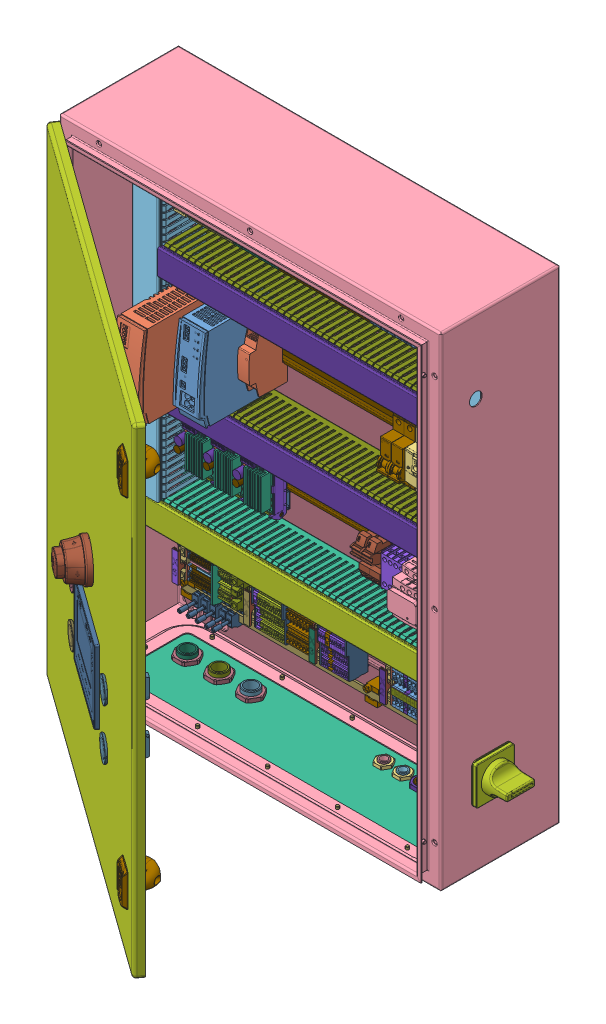
SolidWorks assembly Armoir életrique v46.step, configuration Valor predeterminado. Lengths in mm.
Overall size (649.87 789 553.64).
1537 component instances, 158 part files, 0 mates.
Components (placement in the parent):
- EM-241C_v4.step-1: EM-241C_v4.step [Valor predeterminado] at (-459.7091 5.608 81.2521) size (46 89.6 55.6)
  - DesignRootModel.step-1: DesignRootModel.step [Valor predeterminado] at origin size (42 72 25.9)
    - Submodel-BC846_SOT23_NPN-65V-0.1A_part_simplified_SOT23.step-1: Submodel-BC846_SOT23_NPN-65V-0.1A_part_simplified_SOT23.step [Valor predeterminado] at (643.2091 273.9352 -25.8521) size (3 2.5 1.1)
      - Submodel-C_UsersTino Hellbergworks3D kokeilujaEM-241Cver4_PCB3DInput_SOT-23.xtd.step-1: Submodel-C_UsersTino Hellbergworks3D kokeilujaEM-241Cver4_PCB3DInput_SOT-23.xtd.step [Valor predeterminado] at (0 0.1143 0.55) x (-1 0 0) z (0 1 0) size (3 1.1 2.5)
        - SOT-23.step-1: SOT-23.step [Valor predeterminado] at origin size (3 1.1 2.5)
    - Submodel-BC846_SOT23_NPN-65V-0.1A_part_simplified_SOT23_1.step-1: Submodel-BC846_SOT23_NPN-65V-0.1A_part_simplified_SOT23_1.step [Valor predeterminado] at (643.2091 292.4352 -25.8521) x (0 1 0) z (0 0 1) size (3 2.5 1.1)
      - Submodel-C_UsersTino Hellbergworks3D kokeilujaEM-241Cver4_PCB3DInput_SOT-23.xtd_1.step-1: Submodel-C_UsersTino Hellbergworks3D kokeilujaEM-241Cver4_PCB3DInput_SOT-23.xtd_1.step [Valor predeterminado] at (0 0.1143 0.55) x (-1 0 0) z (0 1 0) size (3 1.1 2.5)
        - SOT-23.step-1: SOT-23.step [Valor predeterminado] at origin size (3 1.1 2.5)
    - Submodel-MMUN2211LT1_SOT23_NPN-50V-0.1A-DIGI_part_simplified_SOT23.step-1: Submodel-MMUN2211LT1_SOT23_NPN-50V-0.1A-DIGI_part_simplified_SOT23.step [Valor predeterminado] at (653.9591 261.1852 -25.8521) size (3 2.5 1.1)
      - Submodel-C_UsersTino Hellbergworks3D kokeilujaEM-241Cver4_PCB3DInput_SOT-23.xtd_2.step-1: Submodel-C_UsersTino Hellbergworks3D kokeilujaEM-241Cver4_PCB3DInput_SOT-23.xtd_2.step [Valor predeterminado] at (0 0.1143 0.55) x (-1 0 0) z (0 1 0) size (3 1.1 2.5)
        - SOT-23.step-1: SOT-23.step [Valor predeterminado] at origin size (3 1.1 2.5)
    - Submodel-RES0805_10R_part_simplified_0805.step-1: Submodel-RES0805_10R_part_simplified_0805.step [Valor predeterminado] at (622.4591 268.6852 -25.8521) x (0 -1 0) z (0 0 1) size (2 1.25 0.6)
      - Submodel-C_UsersTino Hellbergworks3D kokeilujaEM-241Cver4_PCB3DInput_SRES 0805.xtd.step-1: Submodel-C_UsersTino Hellbergworks3D kokeilujaEM-241Cver4_PCB3DInput_SRES 0805.xtd.step [Valor predeterminado] at (-0.975 -0.625 0.025) x (1 0 0) z (0 -1 0) size (2 0.6 1.25)
        - RES 0805.step-1: RES 0805.step [Valor predeterminado] at origin size (2 0.6 1.25)
    - Submodel-RES0805_3K9_part_simplified_0805.step-1: Submodel-RES0805_3K9_part_simplified_0805.step [Valor predeterminado] at (633.7091 264.9352 -25.8521) x (-1 0 0) z (0 0 1) size (2 1.25 0.6)
      - Submodel-C_UsersTino Hellbergworks3D kokeilujaEM-241Cver4_PCB3DInput_SRES 0805.xtd_1.step-1: Submodel-C_UsersTino Hellbergworks3D kokeilujaEM-241Cver4_PCB3DInput_SRES 0805.xtd_1.step [Valor predeterminado] at (-0.975 -0.625 0.025) x (1 0 0) z (0 -1 0) size (2 0.6 1.25)
        - RES 0805.step-1: RES 0805.step [Valor predeterminado] at origin size (2 0.6 1.25)
    - Submodel-RES0805_22K_part_simplified_0805.step-1: Submodel-RES0805_22K_part_simplified_0805.step [Valor predeterminado] at (641.9591 252.4352 -25.8521) x (0 1 0) z (0 0 1) size (2 1.25 0.6)
      - Submodel-C_UsersTino Hellbergworks3D kokeilujaEM-241Cver4_PCB3DInput_SRES 0805.xtd_2.step-1: Submodel-C_UsersTino Hellbergworks3D kokeilujaEM-241Cver4_PCB3DInput_SRES 0805.xtd_2.step [Valor predeterminado] at (-0.975 -0.625 0.025) x (1 0 0) z (0 -1 0) size (2 0.6 1.25)
        - RES 0805.step-1: RES 0805.step [Valor predeterminado] at origin size (2 0.6 1.25)
    - Submodel-RES0805_22K_part_simplified_0805_1.step-1: Submodel-RES0805_22K_part_simplified_0805_1.step [Valor predeterminado] at (633.7091 263.1852 -25.8521) x (-1 0 0) z (0 0 1) size (2 1.25 0.6)
      - Submodel-C_UsersTino Hellbergworks3D kokeilujaEM-241Cver4_PCB3DInput_SRES 0805.xtd_3.step-1: Submodel-C_UsersTino Hellbergworks3D kokeilujaEM-241Cver4_PCB3DInput_SRES 0805.xtd_3.step [Valor predeterminado] at (-0.975 -0.625 0.025) x (1 0 0) z (0 -1 0) size (2 0.6 1.25)
        - RES 0805.step-1: RES 0805.step [Valor predeterminado] at origin size (2 0.6 1.25)
    - Submodel-RES0805_1K2_part_simplified_0805.step-1: Submodel-RES0805_1K2_part_simplified_0805.step [Valor predeterminado] at (633.7091 266.6852 -25.8521) x (-1 0 0) z (0 0 1) size (2 1.25 0.6)
      - Submodel-C_UsersTino Hellbergworks3D kokeilujaEM-241Cver4_PCB3DInput_SRES 0805.xtd_4.step-1: Submodel-C_UsersTino Hellbergworks3D kokeilujaEM-241Cver4_PCB3DInput_SRES 0805.xtd_4.step [Valor predeterminado] at (-0.975 -0.625 0.025) x (1 0 0) z (0 -1 0) size (2 0.6 1.25)
        - RES 0805.step-1: RES 0805.step [Valor predeterminado] at origin size (2 0.6 1.25)
    - Submodel-RES0805_1K2_part_simplified_0805_1.step-1: Submodel-RES0805_1K2_part_simplified_0805_1.step [Valor predeterminado] at (634.2091 293.1852 -25.8521) x (-1 0 0) z (0 0 1) size (2 1.25 0.6)
      - Submodel-C_UsersTino Hellbergworks3D kokeilujaEM-241Cver4_PCB3DInput_SRES 0805.xtd_5.step-1: Submodel-C_UsersTino Hellbergworks3D kokeilujaEM-241Cver4_PCB3DInput_SRES 0805.xtd_5.step [Valor predeterminado] at (-0.975 -0.625 0.025) x (1 0 0) z (0 -1 0) size (2 0.6 1.25)
        - RES 0805.step-1: RES 0805.step [Valor predeterminado] at origin size (2 0.6 1.25)
    - Submodel-RES0805_47K_part_simplified_0805.step-1: Submodel-RES0805_47K_part_simplified_0805.step [Valor predeterminado] at (656.4591 267.1852 -25.8521) x (-1 0 0) z (0 0 1) size (2 1.25 0.6)
      - Submodel-C_UsersTino Hellbergworks3D kokeilujaEM-241Cver4_PCB3DInput_SRES 0805.xtd_6.step-1: Submodel-C_UsersTino Hellbergworks3D kokeilujaEM-241Cver4_PCB3DInput_SRES 0805.xtd_6.step [Valor predeterminado] at (-0.975 -0.625 0.025) x (1 0 0) z (0 -1 0) size (2 0.6 1.25)
        - RES 0805.step-1: RES 0805.step [Valor predeterminado] at origin size (2 0.6 1.25)
    - Submodel-RES0805_47K_part_simplified_0805_1.step-1: Submodel-RES0805_47K_part_simplified_0805_1.step [Valor predeterminado] at (626.7091 257.1852 -25.8521) size (2 1.25 0.6)
      - Submodel-C_UsersTino Hellbergworks3D kokeilujaEM-241Cver4_PCB3DInput_SRES 0805.xtd_7.step-1: Submodel-C_UsersTino Hellbergworks3D kokeilujaEM-241Cver4_PCB3DInput_SRES 0805.xtd_7.step [Valor predeterminado] at (-0.975 -0.625 0.025) x (1 0 0) z (0 -1 0) size (2 0.6 1.25)
        - RES 0805.step-1: RES 0805.step [Valor predeterminado] at origin size (2 0.6 1.25)
    - Submodel-RES0805_47K_part_simplified_0805_2.step-1: Submodel-RES0805_47K_part_simplified_0805_2.step [Valor predeterminado] at (626.2091 253.4352 -25.8521) x (-1 0 0) z (0 0 1) size (2 1.25 0.6)
      - Submodel-C_UsersTino Hellbergworks3D kokeilujaEM-241Cver4_PCB3DInput_SRES 0805.xtd_8.step-1: Submodel-C_UsersTino Hellbergworks3D kokeilujaEM-241Cver4_PCB3DInput_SRES 0805.xtd_8.step [Valor predeterminado] at (-0.975 -0.625 0.025) x (1 0 0) z (0 -1 0) size (2 0.6 1.25)
        - RES 0805.step-1: RES 0805.step [Valor predeterminado] at origin size (2 0.6 1.25)
    - Submodel-RES0805_47K_part_simplified_0805_3.step-1: Submodel-RES0805_47K_part_simplified_0805_3.step [Valor predeterminado] at (626.2091 251.4352 -25.8521) x (-1 0 0) z (0 0 1) size (2 1.25 0.6)
      - Submodel-C_UsersTino Hellbergworks3D kokeilujaEM-241Cver4_PCB3DInput_SRES 0805.xtd_9.step-1: Submodel-C_UsersTino Hellbergworks3D kokeilujaEM-241Cver4_PCB3DInput_SRES 0805.xtd_9.step [Valor predeterminado] at (-0.975 -0.625 0.025) x (1 0 0) z (0 -1 0) size (2 0.6 1.25)
        - RES 0805.step-1: RES 0805.step [Valor predeterminado] at origin size (2 0.6 1.25)
    - Submodel-RES0805_47K_part_simplified_0805_4.step-1: Submodel-RES0805_47K_part_simplified_0805_4.step [Valor predeterminado] at (630.2091 257.1852 -25.8521) size (2 1.25 0.6)
      - Submodel-C_UsersTino Hellbergworks3D kokeilujaEM-241Cver4_PCB3DInput_SRES 0805.xtd_10.step-1: Submodel-C_UsersTino Hellbergworks3D kokeilujaEM-241Cver4_PCB3DInput_SRES 0805.xtd_10.step [Valor predeterminado] at (-0.975 -0.625 0.025) x (1 0 0) z (0 -1 0) size (2 0.6 1.25)
        - RES 0805.step-1: RES 0805.step [Valor predeterminado] at origin size (2 0.6 1.25)
    - Submodel-RES0805_47K_part_simplified_0805_5.step-1: Submodel-RES0805_47K_part_simplified_0805_5.step [Valor predeterminado] at (629.9591 253.4352 -25.8521) x (-1 0 0) z (0 0 1) size (2 1.25 0.6)
      - Submodel-C_UsersTino Hellbergworks3D kokeilujaEM-241Cver4_PCB3DInput_SRES 0805.xtd_11.step-1: Submodel-C_UsersTino Hellbergworks3D kokeilujaEM-241Cver4_PCB3DInput_SRES 0805.xtd_11.step [Valor predeterminado] at (-0.975 -0.625 0.025) x (1 0 0) z (0 -1 0) size (2 0.6 1.25)
        - RES 0805.step-1: RES 0805.step [Valor predeterminado] at origin size (2 0.6 1.25)
    - Submodel-RES0805_47K_part_simplified_0805_6.step-1: Submodel-RES0805_47K_part_simplified_0805_6.step [Valor predeterminado] at (629.9591 251.4352 -25.8521) x (-1 0 0) z (0 0 1) size (2 1.25 0.6)
      - Submodel-C_UsersTino Hellbergworks3D kokeilujaEM-241Cver4_PCB3DInput_SRES 0805.xtd_12.step-1: Submodel-C_UsersTino Hellbergworks3D kokeilujaEM-241Cver4_PCB3DInput_SRES 0805.xtd_12.step [Valor predeterminado] at (-0.975 -0.625 0.025) x (1 0 0) z (0 -1 0) size (2 0.6 1.25)
        - RES 0805.step-1: RES 0805.step [Valor predeterminado] at origin size (2 0.6 1.25)
    - Submodel-RES0805_47K_part_simplified_0805_7.step-1: Submodel-RES0805_47K_part_simplified_0805_7.step [Valor predeterminado] at (634.4591 256.4352 -25.8521) x (0 1 0) z (0 0 1) size (2 1.25 0.6)
      - Submodel-C_UsersTino Hellbergworks3D kokeilujaEM-241Cver4_PCB3DInput_SRES 0805.xtd_13.step-1: Submodel-C_UsersTino Hellbergworks3D kokeilujaEM-241Cver4_PCB3DInput_SRES 0805.xtd_13.step [Valor predeterminado] at (-0.975 -0.625 0.025) x (1 0 0) z (0 -1 0) size (2 0.6 1.25)
        - RES 0805.step-1: RES 0805.step [Valor predeterminado] at origin size (2 0.6 1.25)
    - Submodel-RES0805_47K_part_simplified_0805_8.step-1: Submodel-RES0805_47K_part_simplified_0805_8.step [Valor predeterminado] at (633.7091 253.4352 -25.8521) x (-1 0 0) z (0 0 1) size (2 1.25 0.6)
      - Submodel-C_UsersTino Hellbergworks3D kokeilujaEM-241Cver4_PCB3DInput_SRES 0805.xtd_14.step-1: Submodel-C_UsersTino Hellbergworks3D kokeilujaEM-241Cver4_PCB3DInput_SRES 0805.xtd_14.step [Valor predeterminado] at (-0.975 -0.625 0.025) x (1 0 0) z (0 -1 0) size (2 0.6 1.25)
        - RES 0805.step-1: RES 0805.step [Valor predeterminado] at origin size (2 0.6 1.25)
    - Submodel-RES0805_47K_part_simplified_0805_9.step-1: Submodel-RES0805_47K_part_simplified_0805_9.step [Valor predeterminado] at (633.7091 251.4352 -25.8521) x (-1 0 0) z (0 0 1) size (2 1.25 0.6)
      - Submodel-C_UsersTino Hellbergworks3D kokeilujaEM-241Cver4_PCB3DInput_SRES 0805.xtd_15.step-1: Submodel-C_UsersTino Hellbergworks3D kokeilujaEM-241Cver4_PCB3DInput_SRES 0805.xtd_15.step [Valor predeterminado] at (-0.975 -0.625 0.025) x (1 0 0) z (0 -1 0) size (2 0.6 1.25)
        - RES 0805.step-1: RES 0805.step [Valor predeterminado] at origin size (2 0.6 1.25)
    - Submodel-RES0805_47K_part_simplified_0805_10.step-1: Submodel-RES0805_47K_part_simplified_0805_10.step [Valor predeterminado] at (639.7091 255.6852 -25.8521) size (2 1.25 0.6)
      - Submodel-C_UsersTino Hellbergworks3D kokeilujaEM-241Cver4_PCB3DInput_SRES 0805.xtd_16.step-1: Submodel-C_UsersTino Hellbergworks3D kokeilujaEM-241Cver4_PCB3DInput_SRES 0805.xtd_16.step [Valor predeterminado] at (-0.975 -0.625 0.025) x (1 0 0) z (0 -1 0) size (2 0.6 1.25)
        - RES 0805.step-1: RES 0805.step [Valor predeterminado] at origin size (2 0.6 1.25)
    - Submodel-RES0805_47K_part_simplified_0805_11.step-1: Submodel-RES0805_47K_part_simplified_0805_11.step [Valor predeterminado] at (637.4591 253.4352 -25.8521) size (2 1.25 0.6)
      - Submodel-C_UsersTino Hellbergworks3D kokeilujaEM-241Cver4_PCB3DInput_SRES 0805.xtd_17.step-1: Submodel-C_UsersTino Hellbergworks3D kokeilujaEM-241Cver4_PCB3DInput_SRES 0805.xtd_17.step [Valor predeterminado] at (-0.975 -0.625 0.025) x (1 0 0) z (0 -1 0) size (2 0.6 1.25)
        - RES 0805.step-1: RES 0805.step [Valor predeterminado] at origin size (2 0.6 1.25)
    - Submodel-RES0805_47K_part_simplified_0805_12.step-1: Submodel-RES0805_47K_part_simplified_0805_12.step [Valor predeterminado] at (637.4591 251.4352 -25.8521) size (2 1.25 0.6)
      - Submodel-C_UsersTino Hellbergworks3D kokeilujaEM-241Cver4_PCB3DInput_SRES 0805.xtd_18.step-1: Submodel-C_UsersTino Hellbergworks3D kokeilujaEM-241Cver4_PCB3DInput_SRES 0805.xtd_18.step [Valor predeterminado] at (-0.975 -0.625 0.025) x (1 0 0) z (0 -1 0) size (2 0.6 1.25)
        - RES 0805.step-1: RES 0805.step [Valor predeterminado] at origin size (2 0.6 1.25)
    - Submodel-RES0805_47K_part_simplified_0805_13.step-1: Submodel-RES0805_47K_part_simplified_0805_13.step [Valor predeterminado] at (657.4591 258.6852 -25.8521) x (-1 0 0) z (0 0 1) size (2 1.25 0.6)
      - Submodel-C_UsersTino Hellbergworks3D kokeilujaEM-241Cver4_PCB3DInput_SRES 0805.xtd_19.step-1: Submodel-C_UsersTino Hellbergworks3D kokeilujaEM-241Cver4_PCB3DInput_SRES 0805.xtd_19.step [Valor predeterminado] at (-0.975 -0.625 0.025) x (1 0 0) z (0 -1 0) size (2 0.6 1.25)
        - RES 0805.step-1: RES 0805.step [Valor predeterminado] at origin size (2 0.6 1.25)
    - Submodel-RES0805_1M_part_simplified_0805.step-1: Submodel-RES0805_1M_part_simplified_0805.step [Valor predeterminado] at (641.4591 269.6852 -25.8521) x (0 -1 0) z (0 0 1) size (2 1.25 0.6)
      - Submodel-C_UsersTino Hellbergworks3D kokeilujaEM-241Cver4_PCB3DInput_SRES 0805.xtd_20.step-1: Submodel-C_UsersTino Hellbergworks3D kokeilujaEM-241Cver4_PCB3DInput_SRES 0805.xtd_20.step [Valor predeterminado] at (-0.975 -0.625 0.025) x (1 0 0) z (0 -1 0) size (2 0.6 1.25)
        - RES 0805.step-1: RES 0805.step [Valor predeterminado] at origin size (2 0.6 1.25)
    - Submodel-RES0805_22R_part_simplified_0805.step-1: Submodel-RES0805_22R_part_simplified_0805.step [Valor predeterminado] at (637.9591 293.1852 -25.8521) x (-1 0 0) z (0 0 1) size (2 1.25 0.6)
      - Submodel-C_UsersTino Hellbergworks3D kokeilujaEM-241Cver4_PCB3DInput_SRES 0805.xtd_21.step-1: Submodel-C_UsersTino Hellbergworks3D kokeilujaEM-241Cver4_PCB3DInput_SRES 0805.xtd_21.step [Valor predeterminado] at (-0.975 -0.625 0.025) x (1 0 0) z (0 -1 0) size (2 0.6 1.25)
        - RES 0805.step-1: RES 0805.step [Valor predeterminado] at origin size (2 0.6 1.25)
    - Submodel-RES0805_22R_part_simplified_0805_1.step-1: Submodel-RES0805_22R_part_simplified_0805_1.step [Valor predeterminado] at (643.4591 269.6852 -25.8521) x (0 -1 0) z (0 0 1) size (2 1.25 0.6)
      - Submodel-C_UsersTino Hellbergworks3D kokeilujaEM-241Cver4_PCB3DInput_SRES 0805.xtd_22.step-1: Submodel-C_UsersTino Hellbergworks3D kokeilujaEM-241Cver4_PCB3DInput_SRES 0805.xtd_22.step [Valor predeterminado] at (-0.975 -0.625 0.025) x (1 0 0) z (0 -1 0) size (2 0.6 1.25)
        - RES 0805.step-1: RES 0805.step [Valor predeterminado] at origin size (2 0.6 1.25)
    - Submodel-RES0805_100K_part_simplified_0805.step-1: Submodel-RES0805_100K_part_simplified_0805.step [Valor predeterminado] at (653.9591 258.6852 -25.8521) x (-1 0 0) z (0 0 1) size (2 1.25 0.6)
      - Submodel-C_UsersTino Hellbergworks3D kokeilujaEM-241Cver4_PCB3DInput_SRES 0805.xtd_23.step-1: Submodel-C_UsersTino Hellbergworks3D kokeilujaEM-241Cver4_PCB3DInput_SRES 0805.xtd_23.step [Valor predeterminado] at (-0.975 -0.625 0.025) x (1 0 0) z (0 -1 0) size (2 0.6 1.25)
        - RES 0805.step-1: RES 0805.step [Valor predeterminado] at origin size (2 0.6 1.25)
    - Submodel-RES0805_100K_part_simplified_0805_1.step-1: Submodel-RES0805_100K_part_simplified_0805_1.step [Valor predeterminado] at (640.7091 273.6852 -25.8521) x (0 1 0) z (0 0 1) size (2 1.25 0.6)
      - Submodel-C_UsersTino Hellbergworks3D kokeilujaEM-241Cver4_PCB3DInput_SRES 0805.xtd_24.step-1: Submodel-C_UsersTino Hellbergworks3D kokeilujaEM-241Cver4_PCB3DInput_SRES 0805.xtd_24.step [Valor predeterminado] at (-0.975 -0.625 0.025) x (1 0 0) z (0 -1 0) size (2 0.6 1.25)
        - RES 0805.step-1: RES 0805.step [Valor predeterminado] at origin size (2 0.6 1.25)
    - Submodel-RES0805_100K_part_simplified_0805_2.step-1: Submodel-RES0805_100K_part_simplified_0805_2.step [Valor predeterminado] at (637.9591 290.9352 -25.8521) size (2 1.25 0.6)
      - Submodel-C_UsersTino Hellbergworks3D kokeilujaEM-241Cver4_PCB3DInput_SRES 0805.xtd_25.step-1: Submodel-C_UsersTino Hellbergworks3D kokeilujaEM-241Cver4_PCB3DInput_SRES 0805.xtd_25.step [Valor predeterminado] at (-0.975 -0.625 0.025) x (1 0 0) z (0 -1 0) size (2 0.6 1.25)
        - RES 0805.step-1: RES 0805.step [Valor predeterminado] at origin size (2 0.6 1.25)
    - Submodel-RES0805_100K_part_simplified_0805_3.step-1: Submodel-RES0805_100K_part_simplified_0805_3.step [Valor predeterminado] at (620.7091 268.6852 -25.8521) x (0 -1 0) z (0 0 1) size (2 1.25 0.6)
      - Submodel-C_UsersTino Hellbergworks3D kokeilujaEM-241Cver4_PCB3DInput_SRES 0805.xtd_26.step-1: Submodel-C_UsersTino Hellbergworks3D kokeilujaEM-241Cver4_PCB3DInput_SRES 0805.xtd_26.step [Valor predeterminado] at (-0.975 -0.625 0.025) x (1 0 0) z (0 -1 0) size (2 0.6 1.25)
        - RES 0805.step-1: RES 0805.step [Valor predeterminado] at origin size (2 0.6 1.25)
    - Submodel-RES0805_100K_part_simplified_0805_4.step-1: Submodel-RES0805_100K_part_simplified_0805_4.step [Valor predeterminado] at (627.9591 262.9352 -25.8521) x (0 1 0) z (0 0 1) size (2 1.25 0.6)
      - Submodel-C_UsersTino Hellbergworks3D kokeilujaEM-241Cver4_PCB3DInput_SRES 0805.xtd_27.step-1: Submodel-C_UsersTino Hellbergworks3D kokeilujaEM-241Cver4_PCB3DInput_SRES 0805.xtd_27.step [Valor predeterminado] at (-0.975 -0.625 0.025) x (1 0 0) z (0 -1 0) size (2 0.6 1.25)
        - RES 0805.step-1: RES 0805.step [Valor predeterminado] at origin size (2 0.6 1.25)
    - Submodel-RES0805_100K_part_simplified_0805_5.step-1: Submodel-RES0805_100K_part_simplified_0805_5.step [Valor predeterminado] at (653.4591 251.9352 -25.8521) x (0 -1 0) z (0 0 1) size (2 1.25 0.6)
      - Submodel-C_UsersTino Hellbergworks3D kokeilujaEM-241Cver4_PCB3DInput_SRES 0805.xtd_28.step-1: Submodel-C_UsersTino Hellbergworks3D kokeilujaEM-241Cver4_PCB3DInput_SRES 0805.xtd_28.step [Valor predeterminado] at (-0.975 -0.625 0.025) x (1 0 0) z (0 -1 0) size (2 0.6 1.25)
        - RES 0805.step-1: RES 0805.step [Valor predeterminado] at origin size (2 0.6 1.25)
    - Submodel-RES0805_100K_part_simplified_0805_6.step-1: Submodel-RES0805_100K_part_simplified_0805_6.step [Valor predeterminado] at (640.2091 252.4352 -25.8521) x (0 1 0) z (0 0 1) size (2 1.25 0.6)
      - Submodel-C_UsersTino Hellbergworks3D kokeilujaEM-241Cver4_PCB3DInput_SRES 0805.xtd_29.step-1: Submodel-C_UsersTino Hellbergworks3D kokeilujaEM-241Cver4_PCB3DInput_SRES 0805.xtd_29.step [Valor predeterminado] at (-0.975 -0.625 0.025) x (1 0 0) z (0 -1 0) size (2 0.6 1.25)
        - RES 0805.step-1: RES 0805.step [Valor predeterminado] at origin size (2 0.6 1.25)
    - Submodel-RES0805_10K_part_simplified_0805.step-1: Submodel-RES0805_10K_part_simplified_0805.step [Valor predeterminado] at (657.4591 252.9352 -25.8521) x (-1 0 0) z (0 0 1) size (2 1.25 0.6)
      - Submodel-C_UsersTino Hellbergworks3D kokeilujaEM-241Cver4_PCB3DInput_SRES 0805.xtd_30.step-1: Submodel-C_UsersTino Hellbergworks3D kokeilujaEM-241Cver4_PCB3DInput_SRES 0805.xtd_30.step [Valor predeterminado] at (-0.975 -0.625 0.025) x (1 0 0) z (0 -1 0) size (2 0.6 1.25)
        - RES 0805.step-1: RES 0805.step [Valor predeterminado] at origin size (2 0.6 1.25)
    - Submodel-RES0805_10K_part_simplified_0805_1.step-1: Submodel-RES0805_10K_part_simplified_0805_1.step [Valor predeterminado] at (657.4591 262.1852 -25.8521) size (2 1.25 0.6)
      - Submodel-C_UsersTino Hellbergworks3D kokeilujaEM-241Cver4_PCB3DInput_SRES 0805.xtd_31.step-1: Submodel-C_UsersTino Hellbergworks3D kokeilujaEM-241Cver4_PCB3DInput_SRES 0805.xtd_31.step [Valor predeterminado] at (-0.975 -0.625 0.025) x (1 0 0) z (0 -1 0) size (2 0.6 1.25)
        - RES 0805.step-1: RES 0805.step [Valor predeterminado] at origin size (2 0.6 1.25)
    - Submodel-RES0805_10K_part_simplified_0805_2.step-1: Submodel-RES0805_10K_part_simplified_0805_2.step [Valor predeterminado] at (657.4591 260.4352 -25.8521) size (2 1.25 0.6)
      - Submodel-C_UsersTino Hellbergworks3D kokeilujaEM-241Cver4_PCB3DInput_SRES 0805.xtd_32.step-1: Submodel-C_UsersTino Hellbergworks3D kokeilujaEM-241Cver4_PCB3DInput_SRES 0805.xtd_32.step [Valor predeterminado] at (-0.975 -0.625 0.025) x (1 0 0) z (0 -1 0) size (2 0.6 1.25)
        - RES 0805.step-1: RES 0805.step [Valor predeterminado] at origin size (2 0.6 1.25)
    - Submodel-RES0805_10K_part_simplified_0805_3.step-1: Submodel-RES0805_10K_part_simplified_0805_3.step [Valor predeterminado] at (646.7091 252.4352 -25.8521) x (0 1 0) z (0 0 1) size (2 1.25 0.6)
      - Submodel-C_UsersTino Hellbergworks3D kokeilujaEM-241Cver4_PCB3DInput_SRES 0805.xtd_33.step-1: Submodel-C_UsersTino Hellbergworks3D kokeilujaEM-241Cver4_PCB3DInput_SRES 0805.xtd_33.step [Valor predeterminado] at (-0.975 -0.625 0.025) x (1 0 0) z (0 -1 0) size (2 0.6 1.25)
        - RES 0805.step-1: RES 0805.step [Valor predeterminado] at origin size (2 0.6 1.25)
    - Submodel-RES1206_10R_part_simplified_1206.step-1: Submodel-RES1206_10R_part_simplified_1206.step [Valor predeterminado] at (650.9591 248.6852 -25.8521) size (3.35 1.73 0.85)
      - Submodel-C_UsersTino Hellbergworks3D kokeilujaEM-241Cver4_PCB3DInput_SRES-1206.xtd.step-1: Submodel-C_UsersTino Hellbergworks3D kokeilujaEM-241Cver4_PCB3DInput_SRES-1206.xtd.step [Valor predeterminado] x (1 0 0) z (0 -1 0) size (3.35 0.85 1.73)
        - RES-1206.step-1: RES-1206.step [Valor predeterminado] at origin size (3.35 0.85 1.73)
    - Submodel-RES0805_1K_part_simplified_0805.step-1: Submodel-RES0805_1K_part_simplified_0805.step [Valor predeterminado] at (657.4591 251.1852 -25.8521) x (-1 0 0) z (0 0 1) size (2 1.25 0.6)
      - Submodel-C_UsersTino Hellbergworks3D kokeilujaEM-241Cver4_PCB3DInput_SRES 0805.xtd_34.step-1: Submodel-C_UsersTino Hellbergworks3D kokeilujaEM-241Cver4_PCB3DInput_SRES 0805.xtd_34.step [Valor predeterminado] at (-0.975 -0.625 0.025) x (1 0 0) z (0 -1 0) size (2 0.6 1.25)
        - RES 0805.step-1: RES 0805.step [Valor predeterminado] at origin size (2 0.6 1.25)
    - Submodel-RES0805_1K_part_simplified_0805_1.step-1: Submodel-RES0805_1K_part_simplified_0805_1.step [Valor predeterminado] at (650.9591 273.4352 -25.8521) x (0 1 0) z (0 0 1) size (2 1.25 0.6)
      - Submodel-C_UsersTino Hellbergworks3D kokeilujaEM-241Cver4_PCB3DInput_SRES 0805.xtd_35.step-1: Submodel-C_UsersTino Hellbergworks3D kokeilujaEM-241Cver4_PCB3DInput_SRES 0805.xtd_35.step [Valor predeterminado] at (-0.975 -0.625 0.025) x (1 0 0) z (0 -1 0) size (2 0.6 1.25)
        - RES 0805.step-1: RES 0805.step [Valor predeterminado] at origin size (2 0.6 1.25)
    - Submodel-RES1206_100R_part_simplified_1206.step-1: Submodel-RES1206_100R_part_simplified_1206.step [Valor predeterminado] at (650.2091 252.4352 -25.8521) x (0 1 0) z (0 0 1) size (3.35 1.73 0.85)
      - Submodel-C_UsersTino Hellbergworks3D kokeilujaEM-241Cver4_PCB3DInput_SRES-1206.xtd_1.step-1: Submodel-C_UsersTino Hellbergworks3D kokeilujaEM-241Cver4_PCB3DInput_SRES-1206.xtd_1.step [Valor predeterminado] x (1 0 0) z (0 -1 0) size (3.35 0.85 1.73)
        - RES-1206.step-1: RES-1206.step [Valor predeterminado] at origin size (3.35 0.85 1.73)
    - Submodel-RES0805_220R_part_simplified_0805.step-1: Submodel-RES0805_220R_part_simplified_0805.step [Valor predeterminado] at (657.4591 273.9352 -25.8521) x (0 1 0) z (0 0 1) size (2 1.25 0.6)
      - Submodel-C_UsersTino Hellbergworks3D kokeilujaEM-241Cver4_PCB3DInput_SRES 0805.xtd_36.step-1: Submodel-C_UsersTino Hellbergworks3D kokeilujaEM-241Cver4_PCB3DInput_SRES 0805.xtd_36.step [Valor predeterminado] at (-0.975 -0.625 0.025) x (1 0 0) z (0 -1 0) size (2 0.6 1.25)
        - RES 0805.step-1: RES 0805.step [Valor predeterminado] at origin size (2 0.6 1.25)
    - Submodel-RES0805_220R_part_simplified_0805_1.step-1: Submodel-RES0805_220R_part_simplified_0805_1.step [Valor predeterminado] at (655.4591 273.9352 -25.8521) x (0 1 0) z (0 0 1) size (2 1.25 0.6)
      - Submodel-C_UsersTino Hellbergworks3D kokeilujaEM-241Cver4_PCB3DInput_SRES 0805.xtd_37.step-1: Submodel-C_UsersTino Hellbergworks3D kokeilujaEM-241Cver4_PCB3DInput_SRES 0805.xtd_37.step [Valor predeterminado] at (-0.975 -0.625 0.025) x (1 0 0) z (0 -1 0) size (2 0.6 1.25)
        - RES 0805.step-1: RES 0805.step [Valor predeterminado] at origin size (2 0.6 1.25)
    - Submodel-RES0805_2K2_part_simplified_0805.step-1: Submodel-RES0805_2K2_part_simplified_0805.step [Valor predeterminado] at (618.9591 268.6852 -25.8521) x (0 -1 0) z (0 0 1) size (2 1.25 0.6)
      - Submodel-C_UsersTino Hellbergworks3D kokeilujaEM-241Cver4_PCB3DInput_SRES 0805.xtd_38.step-1: Submodel-C_UsersTino Hellbergworks3D kokeilujaEM-241Cver4_PCB3DInput_SRES 0805.xtd_38.step [Valor predeterminado] at (-0.975 -0.625 0.025) x (1 0 0) z (0 -1 0) size (2 0.6 1.25)
        - RES 0805.step-1: RES 0805.step [Valor predeterminado] at origin size (2 0.6 1.25)
    - Submodel-RES0805_2K2_part_simplified_0805_1.step-1: Submodel-RES0805_2K2_part_simplified_0805_1.step [Valor predeterminado] at (644.9591 252.4352 -25.8521) x (0 -1 0) z (0 0 1) size (2 1.25 0.6)
      - Submodel-C_UsersTino Hellbergworks3D kokeilujaEM-241Cver4_PCB3DInput_SRES 0805.xtd_39.step-1: Submodel-C_UsersTino Hellbergworks3D kokeilujaEM-241Cver4_PCB3DInput_SRES 0805.xtd_39.step [Valor predeterminado] at (-0.975 -0.625 0.025) x (1 0 0) z (0 -1 0) size (2 0.6 1.25)
        - RES 0805.step-1: RES 0805.step [Valor predeterminado] at origin size (2 0.6 1.25)
    - Submodel-RES0805_2K2_part_simplified_0805_2.step-1: Submodel-RES0805_2K2_part_simplified_0805_2.step [Valor predeterminado] at (621.2091 248.9352 -25.8521) x (-1 0 0) z (0 0 1) size (2 1.25 0.6)
      - Submodel-C_UsersTino Hellbergworks3D kokeilujaEM-241Cver4_PCB3DInput_SRES 0805.xtd_40.step-1: Submodel-C_UsersTino Hellbergworks3D kokeilujaEM-241Cver4_PCB3DInput_SRES 0805.xtd_40.step [Valor predeterminado] at (-0.975 -0.625 0.025) x (1 0 0) z (0 -1 0) size (2 0.6 1.25)
        - RES 0805.step-1: RES 0805.step [Valor predeterminado] at origin size (2 0.6 1.25)
    - Submodel-RES0805_2K2_part_simplified_0805_3.step-1: Submodel-RES0805_2K2_part_simplified_0805_3.step [Valor predeterminado] at (626.7091 259.4352 -25.8521) x (-1 0 0) z (0 0 1) size (2 1.25 0.6)
      - Submodel-C_UsersTino Hellbergworks3D kokeilujaEM-241Cver4_PCB3DInput_SRES 0805.xtd_41.step-1: Submodel-C_UsersTino Hellbergworks3D kokeilujaEM-241Cver4_PCB3DInput_SRES 0805.xtd_41.step [Valor predeterminado] at (-0.975 -0.625 0.025) x (1 0 0) z (0 -1 0) size (2 0.6 1.25)
        - RES 0805.step-1: RES 0805.step [Valor predeterminado] at origin size (2 0.6 1.25)
    - Submodel-RES0805_2K2_part_simplified_0805_4.step-1: Submodel-RES0805_2K2_part_simplified_0805_4.step [Valor predeterminado] at (652.9591 273.4352 -25.8521) x (0 1 0) z (0 0 1) size (2 1.25 0.6)
      - Submodel-C_UsersTino Hellbergworks3D kokeilujaEM-241Cver4_PCB3DInput_SRES 0805.xtd_42.step-1: Submodel-C_UsersTino Hellbergworks3D kokeilujaEM-241Cver4_PCB3DInput_SRES 0805.xtd_42.step [Valor predeterminado] at (-0.975 -0.625 0.025) x (1 0 0) z (0 -1 0) size (2 0.6 1.25)
        - RES 0805.step-1: RES 0805.step [Valor predeterminado] at origin size (2 0.6 1.25)
    - Submodel-RES0805_2K2_part_simplified_0805_5.step-1: Submodel-RES0805_2K2_part_simplified_0805_5.step [Valor predeterminado] at (655.9591 271.4352 -25.8521) x (-1 0 0) z (0 0 1) size (2 1.25 0.6)
      - Submodel-C_UsersTino Hellbergworks3D kokeilujaEM-241Cver4_PCB3DInput_SRES 0805.xtd_43.step-1: Submodel-C_UsersTino Hellbergworks3D kokeilujaEM-241Cver4_PCB3DInput_SRES 0805.xtd_43.step [Valor predeterminado] at (-0.975 -0.625 0.025) x (1 0 0) z (0 -1 0) size (2 0.6 1.25)
        - RES 0805.step-1: RES 0805.step [Valor predeterminado] at origin size (2 0.6 1.25)
    - Submodel-RES0805_2K2_part_simplified_0805_6.step-1: Submodel-RES0805_2K2_part_simplified_0805_6.step [Valor predeterminado] at (652.4591 245.9352 -25.8521) x (0 1 0) z (0 0 1) size (2 1.25 0.6)
      - Submodel-C_UsersTino Hellbergworks3D kokeilujaEM-241Cver4_PCB3DInput_SRES 0805.xtd_44.step-1: Submodel-C_UsersTino Hellbergworks3D kokeilujaEM-241Cver4_PCB3DInput_SRES 0805.xtd_44.step [Valor predeterminado] at (-0.975 -0.625 0.025) x (1 0 0) z (0 -1 0) size (2 0.6 1.25)
        - RES 0805.step-1: RES 0805.step [Valor predeterminado] at origin size (2 0.6 1.25)
    - Submodel-PTC_1210_0.1A30V_part_simplified_1210.step-1: Submodel-PTC_1210_0.1A30V_part_simplified_1210.step [Valor predeterminado] at (629.9591 279.4352 -25.8521) x (0 -1 0) z (0 0 1) size (3.2 2.5 1.5)
      - Submodel-C_UsersTino Hellbergworks3D kokeilujaEM-241Cver4_PCB3DInput_SV-1210-HD.xtd.step-1: Submodel-C_UsersTino Hellbergworks3D kokeilujaEM-241Cver4_PCB3DInput_SV-1210-HD.xtd.step [Valor predeterminado] at origin size (3.2 2.5 1.5)
        - V-1210-HD.step-1: V-1210-HD.step [Valor predeterminado] at origin size (3.2 2.5 1.5)
    - Submodel-NTC_0805_100K_part_simplified_0805.step-1: Submodel-NTC_0805_100K_part_simplified_0805.step [Valor predeterminado] at (633.7091 261.1852 -25.8521) size (2 1.25 0.6)
      - Submodel-C_UsersTino Hellbergworks3D kokeilujaEM-241Cver4_PCB3DInput_SRES 0805.xtd_45.step-1: Submodel-C_UsersTino Hellbergworks3D kokeilujaEM-241Cver4_PCB3DInput_SRES 0805.xtd_45.step [Valor predeterminado] at (-0.975 -0.625 0.025) x (1 0 0) z (0 -1 0) size (2 0.6 1.25)
        - RES 0805.step-1: RES 0805.step [Valor predeterminado] at origin size (2 0.6 1.25)
    - Submodel-ATMEGA328P-AU_TQFP32_part_simplified_TQFP32.step-1: Submodel-ATMEGA328P-AU_TQFP32_part_simplified_TQFP32.step [Valor predeterminado] at (646.4591 262.4352 -25.8521) x (-1 0 0) z (0 0 1) size (9.02 9.02 1.15)
      - Submodel-C_UsersTino Hellbergworks3D kokeilujaEM-241Cver4_PCB3DInput_STQFP32.xtd.step-1: Submodel-C_UsersTino Hellbergworks3D kokeilujaEM-241Cver4_PCB3DInput_STQFP32.xtd.step [Valor predeterminado] at (0 0 0.1493) x (1 0 0) z (0 -1 0) size (9.02 1.15 9.02)
        - TQFP32.step-1: TQFP32.step [Valor predeterminado] at origin size (9.02 1.15 9.02)
    - Submodel-HS_SK177-50SA_28.0X50.0_7CW_part_simplified_HS-SK177-50SA.step-1: Submodel-HS_SK177-50SA_28.0X50.0_7CW_part_simplified_HS-SK177-50SA.step [Valor predeterminado] at (659.7091 299.9352 -25.8521) x (-1 0 0) z (0 0 1) size (27.94 50 15.24)
      - Submodel-C_UsersTino Hellbergworks3D kokeilujaEM-241Cver4_PCB3DInput_S-SK177-50.xtd.step-1: Submodel-C_UsersTino Hellbergworks3D kokeilujaEM-241Cver4_PCB3DInput_S-SK177-50.xtd.step [Valor predeterminado] at (0.03 -0.5 2.4) size (27.94 50 15.24)
        - PV-SK177-50.step-1: PV-SK177-50.step [Valor predeterminado] at origin size (27.94 50 15.24)
    - Submodel-BZV55-C6V2_ZENER-6.2V-0.5W_part_simplified_SOD80.step-1: Submodel-BZV55-C6V2_ZENER-6.2V-0.5W_part_simplified_SOD80.step [Valor predeterminado] at (630.7091 262.9352 -25.8521) x (0 1 0) z (0 0 1) size (3.7 1.6 1.6)
      - Submodel-C_UsersTino Hellbergworks3D kokeilujaEM-241Cver4_PCB3DInput_SOD80.xtd.step-1: Submodel-C_UsersTino Hellbergworks3D kokeilujaEM-241Cver4_PCB3DInput_SOD80.xtd.step [Valor predeterminado] at (0.03 0 0) size (3.7 1.6 1.6)
        - SOD80.step-1: SOD80.step [Valor predeterminado] at origin size (3.7 1.6 1.6)
    - Submodel-US1J_1A600V_SMA_part_simplified_SMA.step-1: Submodel-US1J_1A600V_SMA_part_simplified_SMA.step [Valor predeterminado] at (638.4591 271.6852 -25.8521) x (0 1 0) z (0 0 1) size (5.2 2.6 2.45)
      - Submodel-C_UsersTino Hellbergworks3D kokeilujaEM-241Cver4_PCB3DInput_SDO-214AC SMA.xtd.step-1: Submodel-C_UsersTino Hellbergworks3D kokeilujaEM-241Cver4_PCB3DInput_SDO-214AC SMA.xtd.step [Valor predeterminado] at (0 0 1.4) x (0 1 0) z (0 0 1) size (2.6 5.2 2.45)
        - DO-214AC SMA.step-1: DO-214AC SMA.step [Valor predeterminado] at origin size (2.6 5.2 2.45)
    - Submodel-BAS70-04W_0.07A70V-DUAL-SCHOTT_part_simplified_SOT323.step-1: Submodel-BAS70-04W_0.07A70V-DUAL-SCHOTT_part_simplified_SOT323.step [Valor predeterminado] at (642.7091 286.4352 -25.8521) x (0 -1 0) z (0 0 1) size (2.1 2.3 1)
      - Submodel-C_UsersTino Hellbergworks3D kokeilujaEM-241Cver4_PCB3DInput_SOT-323.xtd.step-1: Submodel-C_UsersTino Hellbergworks3D kokeilujaEM-241Cver4_PCB3DInput_SOT-323.xtd.step [Valor predeterminado] at (0 0.0625 0) size (2.1 2.3 1)
        - SOT-323.step-1: SOT-323.step [Valor predeterminado] at origin size (2.1 2.3 1)
    - Submodel-BAS70-04W_0.07A70V-DUAL-SCHOTT_part_simplified_SOT323_1.step-1: Submodel-BAS70-04W_0.07A70V-DUAL-SCHOTT_part_simplified_SOT323_1.step [Valor predeterminado] at (642.7091 278.9352 -25.8521) x (0 -1 0) z (0 0 1) size (2.1 2.3 1)
      - Submodel-C_UsersTino Hellbergworks3D kokeilujaEM-241Cver4_PCB3DInput_SOT-323.xtd_1.step-1: Submodel-C_UsersTino Hellbergworks3D kokeilujaEM-241Cver4_PCB3DInput_SOT-323.xtd_1.step [Valor predeterminado] at (0 0.0625 0) size (2.1 2.3 1)
        - SOT-323.step-1: SOT-323.step [Valor predeterminado] at origin size (2.1 2.3 1)
    - Submodel-LS4148_0.2A100V_SOD80_part_simplified_SOD80.step-1: Submodel-LS4148_0.2A100V_SOD80_part_simplified_SOD80.step [Valor predeterminado] at (651.7091 292.4352 -25.8521) size (3.7 1.6 1.6)
      - Submodel-C_UsersTino Hellbergworks3D kokeilujaEM-241Cver4_PCB3DInput_SOD80.xtd_1.step-1: Submodel-C_UsersTino Hellbergworks3D kokeilujaEM-241Cver4_PCB3DInput_SOD80.xtd_1.step [Valor predeterminado] at (0.03 0 0) size (3.7 1.6 1.6)
        - SOD80.step-1: SOD80.step [Valor predeterminado] at origin size (3.7 1.6 1.6)
    - Submodel-LS4148_0.2A100V_SOD80_part_simplified_SOD80_1.step-1: Submodel-LS4148_0.2A100V_SOD80_part_simplified_SOD80_1.step [Valor predeterminado] at (655.2091 269.4352 -25.8521) size (3.7 1.6 1.6)
      - Submodel-C_UsersTino Hellbergworks3D kokeilujaEM-241Cver4_PCB3DInput_SOD80.xtd_2.step-1: Submodel-C_UsersTino Hellbergworks3D kokeilujaEM-241Cver4_PCB3DInput_SOD80.xtd_2.step [Valor predeterminado] at (0.03 0 0) size (3.7 1.6 1.6)
        - SOD80.step-1: SOD80.step [Valor predeterminado] at origin size (3.7 1.6 1.6)
    - Submodel-TOPLED_RED_645NM180MCD_PLCC2_part_simplified_PLCC2.step-1: Submodel-TOPLED_RED_645NM180MCD_PLCC2_part_simplified_PLCC2.step [Valor predeterminado] at (655.7091 248.6852 -25.8521) x (-1 0 0) z (0 0 1) size (3.5 2.8 1.9)
      - Submodel-C_UsersTino Hellbergworks3D kokeilujaEM-241Cver4_PCB3DInput_SMD LED PLCC-2.xtd.step-1: Submodel-C_UsersTino Hellbergworks3D kokeilujaEM-241Cver4_PCB3DInput_SMD LED PLCC-2.xtd.step [Valor predeterminado] x (0 1 0) z (0 0 -1) size (2.8 3.5 1.9)
        - SMD LED PLCC-2.step-1: SMD LED PLCC-2.step [Valor predeterminado] at origin size (2.8 3.5 1.9)
    - Submodel-CAP1206_10UF_10V_part_simplified_1206.step-1: Submodel-CAP1206_10UF_10V_part_simplified_1206.step [Valor predeterminado] at (654.2091 264.1852 -25.8521) size (3.4 1.8 0.88)
      - Submodel-C_UsersTino Hellbergworks3D kokeilujaEM-241Cver4_PCB3DInput_SCAP 1206.xtd.step-1: Submodel-C_UsersTino Hellbergworks3D kokeilujaEM-241Cver4_PCB3DInput_SCAP 1206.xtd.step [Valor predeterminado] at (97.4085 -43.3809 11.5241) x (1 0 0) z (0 1 0) size (3.4 0.88 1.8)
        - CAP 1206.step-1: CAP 1206.step [Valor predeterminado] at origin size (3.4 0.88 1.8)
    - Submodel-CAP0603_100NF_part_simplified_0603.step-1: Submodel-CAP0603_100NF_part_simplified_0603.step [Valor predeterminado] at (648.4591 252.1852 -25.8521) x (0 1 0) z (0 0 1) size (1.75 0.95 0.87)
      - Submodel-C_UsersTino Hellbergworks3D kokeilujaEM-241Cver4_PCB3DInput_SCAP 0603.xtd.step-1: Submodel-C_UsersTino Hellbergworks3D kokeilujaEM-241Cver4_PCB3DInput_SCAP 0603.xtd.step [Valor predeterminado] at (96.5835 -43.8059 11.5141) x (1 0 0) z (0 1 0) size (1.75 0.87 0.95)
        - CAP 0603.step-1: CAP 0603.step [Valor predeterminado] at origin size (1.75 0.87 0.95)
    - Submodel-CAP0603_100NF_part_simplified_0603_1.step-1: Submodel-CAP0603_100NF_part_simplified_0603_1.step [Valor predeterminado] at (654.9591 252.1852 -25.8521) x (0 -1 0) z (0 0 1) size (1.75 0.95 0.87)
      - Submodel-C_UsersTino Hellbergworks3D kokeilujaEM-241Cver4_PCB3DInput_SCAP 0603.xtd_1.step-1: Submodel-C_UsersTino Hellbergworks3D kokeilujaEM-241Cver4_PCB3DInput_SCAP 0603.xtd_1.step [Valor predeterminado] at (96.5835 -43.8059 11.5141) x (1 0 0) z (0 1 0) size (1.75 0.87 0.95)
        - CAP 0603.step-1: CAP 0603.step [Valor predeterminado] at origin size (1.75 0.87 0.95)
    - Submodel-CAP0603_100NF_part_simplified_0603_2.step-1: Submodel-CAP0603_100NF_part_simplified_0603_2.step [Valor predeterminado] at (653.4591 255.6852 -25.8521) x (0 -1 0) z (0 0 1) size (1.75 0.95 0.87)
      - Submodel-C_UsersTino Hellbergworks3D kokeilujaEM-241Cver4_PCB3DInput_SCAP 0603.xtd_2.step-1: Submodel-C_UsersTino Hellbergworks3D kokeilujaEM-241Cver4_PCB3DInput_SCAP 0603.xtd_2.step [Valor predeterminado] at (96.5835 -43.8059 11.5141) x (1 0 0) z (0 1 0) size (1.75 0.87 0.95)
        - CAP 0603.step-1: CAP 0603.step [Valor predeterminado] at origin size (1.75 0.87 0.95)
    - Submodel-CAP0603_100NF_part_simplified_0603_3.step-1: Submodel-CAP0603_100NF_part_simplified_0603_3.step [Valor predeterminado] at (641.4591 266.1852 -25.8521) size (1.75 0.95 0.87)
      - Submodel-C_UsersTino Hellbergworks3D kokeilujaEM-241Cver4_PCB3DInput_SCAP 0603.xtd_3.step-1: Submodel-C_UsersTino Hellbergworks3D kokeilujaEM-241Cver4_PCB3DInput_SCAP 0603.xtd_3.step [Valor predeterminado] at (96.5835 -43.8059 11.5141) x (1 0 0) z (0 1 0) size (1.75 0.87 0.95)
        - CAP 0603.step-1: CAP 0603.step [Valor predeterminado] at origin size (1.75 0.87 0.95)
    - Submodel-CAP0603_1NF_part_simplified_0603.step-1: Submodel-CAP0603_1NF_part_simplified_0603.step [Valor predeterminado] at (645.2091 277.1852 -25.8521) x (0 1 0) z (0 0 1) size (1.75 0.95 0.87)
      - Submodel-C_UsersTino Hellbergworks3D kokeilujaEM-241Cver4_PCB3DInput_SCAP 0603.xtd_4.step-1: Submodel-C_UsersTino Hellbergworks3D kokeilujaEM-241Cver4_PCB3DInput_SCAP 0603.xtd_4.step [Valor predeterminado] at (96.5835 -43.8059 11.5141) x (1 0 0) z (0 1 0) size (1.75 0.87 0.95)
        - CAP 0603.step-1: CAP 0603.step [Valor predeterminado] at origin size (1.75 0.87 0.95)
    - Submodel-CAP0603_1NF_part_simplified_0603_1.step-1: Submodel-CAP0603_1NF_part_simplified_0603_1.step [Valor predeterminado] at (645.9591 269.6852 -25.8521) x (0 1 0) z (0 0 1) size (1.75 0.95 0.87)
      - Submodel-C_UsersTino Hellbergworks3D kokeilujaEM-241Cver4_PCB3DInput_SCAP 0603.xtd_5.step-1: Submodel-C_UsersTino Hellbergworks3D kokeilujaEM-241Cver4_PCB3DInput_SCAP 0603.xtd_5.step [Valor predeterminado] at (96.5835 -43.8059 11.5141) x (1 0 0) z (0 1 0) size (1.75 0.87 0.95)
        - CAP 0603.step-1: CAP 0603.step [Valor predeterminado] at origin size (1.75 0.87 0.95)
    - Submodel-CAP0603_1NF_part_simplified_0603_2.step-1: Submodel-CAP0603_1NF_part_simplified_0603_2.step [Valor predeterminado] at (638.7091 265.4352 -25.8521) x (0 1 0) z (0 0 1) size (1.75 0.95 0.87)
      - Submodel-C_UsersTino Hellbergworks3D kokeilujaEM-241Cver4_PCB3DInput_SCAP 0603.xtd_6.step-1: Submodel-C_UsersTino Hellbergworks3D kokeilujaEM-241Cver4_PCB3DInput_SCAP 0603.xtd_6.step [Valor predeterminado] at (96.5835 -43.8059 11.5141) x (1 0 0) z (0 1 0) size (1.75 0.87 0.95)
        - CAP 0603.step-1: CAP 0603.step [Valor predeterminado] at origin size (1.75 0.87 0.95)
    - Submodel-CAP0603_1NF_part_simplified_0603_3.step-1: Submodel-CAP0603_1NF_part_simplified_0603_3.step [Valor predeterminado] at (638.7091 261.9352 -25.8521) x (0 1 0) z (0 0 1) size (1.75 0.95 0.87)
      - Submodel-C_UsersTino Hellbergworks3D kokeilujaEM-241Cver4_PCB3DInput_SCAP 0603.xtd_7.step-1: Submodel-C_UsersTino Hellbergworks3D kokeilujaEM-241Cver4_PCB3DInput_SCAP 0603.xtd_7.step [Valor predeterminado] at (96.5835 -43.8059 11.5141) x (1 0 0) z (0 1 0) size (1.75 0.87 0.95)
        - CAP 0603.step-1: CAP 0603.step [Valor predeterminado] at origin size (1.75 0.87 0.95)
    - Submodel-CAP0603_1NF_part_simplified_0603_4.step-1: Submodel-CAP0603_1NF_part_simplified_0603_4.step [Valor predeterminado] at (636.7091 261.9352 -25.8521) x (0 1 0) z (0 0 1) size (1.75 0.95 0.87)
      - Submodel-C_UsersTino Hellbergworks3D kokeilujaEM-241Cver4_PCB3DInput_SCAP 0603.xtd_8.step-1: Submodel-C_UsersTino Hellbergworks3D kokeilujaEM-241Cver4_PCB3DInput_SCAP 0603.xtd_8.step [Valor predeterminado] at (96.5835 -43.8059 11.5141) x (1 0 0) z (0 1 0) size (1.75 0.87 0.95)
        - CAP 0603.step-1: CAP 0603.step [Valor predeterminado] at origin size (1.75 0.87 0.95)
    - Submodel-CAP0603_1NF_part_simplified_0603_5.step-1: Submodel-CAP0603_1NF_part_simplified_0603_5.step [Valor predeterminado] at (636.7091 265.4352 -25.8521) x (0 -1 0) z (0 0 1) size (1.75 0.95 0.87)
      - Submodel-C_UsersTino Hellbergworks3D kokeilujaEM-241Cver4_PCB3DInput_SCAP 0603.xtd_9.step-1: Submodel-C_UsersTino Hellbergworks3D kokeilujaEM-241Cver4_PCB3DInput_SCAP 0603.xtd_9.step [Valor predeterminado] at (96.5835 -43.8059 11.5141) x (1 0 0) z (0 1 0) size (1.75 0.87 0.95)
        - CAP 0603.step-1: CAP 0603.step [Valor predeterminado] at origin size (1.75 0.87 0.95)
    - Submodel-CAP0603_1NF_part_simplified_0603_6.step-1: Submodel-CAP0603_1NF_part_simplified_0603_6.step [Valor predeterminado] at (647.2091 269.6852 -25.8521) x (0 1 0) z (0 0 1) size (1.75 0.95 0.87)
      - Submodel-C_UsersTino Hellbergworks3D kokeilujaEM-241Cver4_PCB3DInput_SCAP 0603.xtd_10.step-1: Submodel-C_UsersTino Hellbergworks3D kokeilujaEM-241Cver4_PCB3DInput_SCAP 0603.xtd_10.step [Valor predeterminado] at (96.5835 -43.8059 11.5141) x (1 0 0) z (0 1 0) size (1.75 0.87 0.95)
        - CAP 0603.step-1: CAP 0603.step [Valor predeterminado] at origin size (1.75 0.87 0.95)
    - Submodel-CAP0603_1NF_part_simplified_0603_7.step-1: Submodel-CAP0603_1NF_part_simplified_0603_7.step [Valor predeterminado] at (645.2091 284.6852 -25.8521) x (0 1 0) z (0 0 1) size (1.75 0.95 0.87)
      - Submodel-C_UsersTino Hellbergworks3D kokeilujaEM-241Cver4_PCB3DInput_SCAP 0603.xtd_11.step-1: Submodel-C_UsersTino Hellbergworks3D kokeilujaEM-241Cver4_PCB3DInput_SCAP 0603.xtd_11.step [Valor predeterminado] at (96.5835 -43.8059 11.5141) x (1 0 0) z (0 1 0) size (1.75 0.87 0.95)
        - CAP 0603.step-1: CAP 0603.step [Valor predeterminado] at origin size (1.75 0.87 0.95)
    - Submodel-CAP0603_2N2_part_simplified_0603.step-1: Submodel-CAP0603_2N2_part_simplified_0603.step [Valor predeterminado] at (645.2091 280.1852 -25.8521) x (0 1 0) z (0 0 1) size (1.75 0.95 0.87)
      - Submodel-C_UsersTino Hellbergworks3D kokeilujaEM-241Cver4_PCB3DInput_SCAP 0603.xtd_12.step-1: Submodel-C_UsersTino Hellbergworks3D kokeilujaEM-241Cver4_PCB3DInput_SCAP 0603.xtd_12.step [Valor predeterminado] at (96.5835 -43.8059 11.5141) x (1 0 0) z (0 1 0) size (1.75 0.87 0.95)
        - CAP 0603.step-1: CAP 0603.step [Valor predeterminado] at origin size (1.75 0.87 0.95)
    - Submodel-CAP0603_2N2_part_simplified_0603_1.step-1: Submodel-CAP0603_2N2_part_simplified_0603_1.step [Valor predeterminado] at (656.9591 285.6852 -25.8521) x (-1 0 0) z (0 0 1) size (1.75 0.95 0.87)
      - Submodel-C_UsersTino Hellbergworks3D kokeilujaEM-241Cver4_PCB3DInput_SCAP 0603.xtd_13.step-1: Submodel-C_UsersTino Hellbergworks3D kokeilujaEM-241Cver4_PCB3DInput_SCAP 0603.xtd_13.step [Valor predeterminado] at (96.5835 -43.8059 11.5141) x (1 0 0) z (0 1 0) size (1.75 0.87 0.95)
        - CAP 0603.step-1: CAP 0603.step [Valor predeterminado] at origin size (1.75 0.87 0.95)
    - Submodel-CAP0603_2N2_part_simplified_0603_2.step-1: Submodel-CAP0603_2N2_part_simplified_0603_2.step [Valor predeterminado] at (645.2091 287.6852 -25.8521) x (0 1 0) z (0 0 1) size (1.75 0.95 0.87)
      - Submodel-C_UsersTino Hellbergworks3D kokeilujaEM-241Cver4_PCB3DInput_SCAP 0603.xtd_14.step-1: Submodel-C_UsersTino Hellbergworks3D kokeilujaEM-241Cver4_PCB3DInput_SCAP 0603.xtd_14.step [Valor predeterminado] at (96.5835 -43.8059 11.5141) x (1 0 0) z (0 1 0) size (1.75 0.87 0.95)
        - CAP 0603.step-1: CAP 0603.step [Valor predeterminado] at origin size (1.75 0.87 0.95)
    - Submodel-CAP0603_2N2_part_simplified_0603_3.step-1: Submodel-CAP0603_2N2_part_simplified_0603_3.step [Valor predeterminado] at (656.7091 278.1852 -25.8521) x (-1 0 0) z (0 0 1) size (1.75 0.95 0.87)
      - Submodel-C_UsersTino Hellbergworks3D kokeilujaEM-241Cver4_PCB3DInput_SCAP 0603.xtd_15.step-1: Submodel-C_UsersTino Hellbergworks3D kokeilujaEM-241Cver4_PCB3DInput_SCAP 0603.xtd_15.step [Valor predeterminado] at (96.5835 -43.8059 11.5141) x (1 0 0) z (0 1 0) size (1.75 0.87 0.95)
